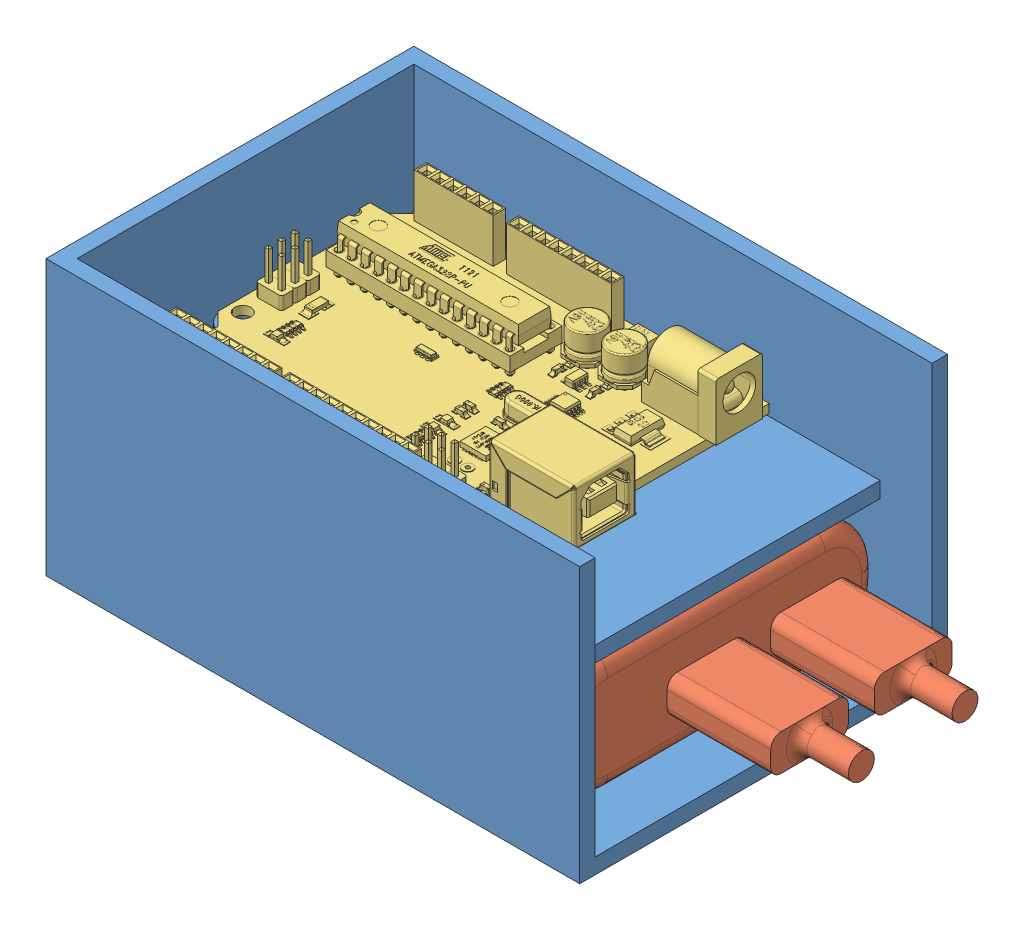
SolidWorks assembly Arduino box assembly, configuration Default. Lengths in mm.
Overall size (123.5 53 71).
3 component instances, 3 part files, 5 mates.
Components (placement in the parent):
- arduino box-1: arduino box [Default] at origin size (103 53 71)
- Power bank-1: Power bank [Default] at (-4.75 0 -0.3741) x (0 0 1) z (-1 0 0) size (62 22.2 120.5)
- arduino uno-1: arduino uno [Default] at (23.04 32.05 -28.04) x (0 0 -1) z (1 0 0) size (53.34 15.25 74.93)
Mates (geometry in assembly coordinates):
- Coincident1: coincident anti-aligned: plane of arduino box-1 through (-50 50 -32.5) normal (1 0 0); plane of Power bank-1 through (-50 22.2 -31.3741) normal (-1 0 0)
- Coincident2: coincident anti-aligned: plane of arduino box-1 through (0 0 0) normal (0 1 0); plane of Power bank-1 through (-4.75 0 -0.3741) normal (0 -1 0)
- Parallel3: parallel aligned: plane of arduino box-1 through (-50 50 -35.5) normal (0 0 -1); plane of arduino uno-1 through (23.04 30.4 -28.04) normal (0 0 -1)
- Coincident8: coincident anti-aligned: plane of arduino box-1 through (7.8 30.4 22.76) normal (0 1 0); plane of arduino uno-1 through (23.04 30.4 -28.04) normal (0 -1 0)
- Concentric1: concentric anti-aligned: cylinder of arduino box-1 through (9.07 30.4 -25.5) axis (0 -1 0) radius 1.6; cylinder of arduino uno-1 through (9.07 30.4 -25.5) axis (0 1 0) radius 1.5875
